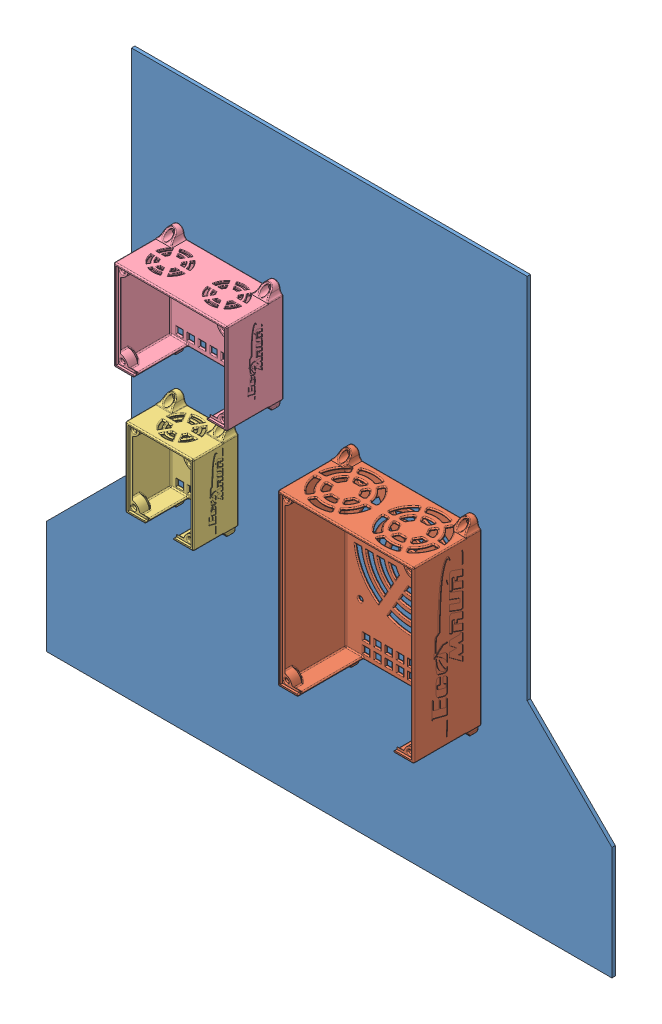
SolidWorks assembly placa_suporte_eletronica_montada, configuration Default. Lengths in mm.
Overall size (500 500 63).
4 component instances, 4 part files, 6 mates.
Components (placement in the parent):
- placa_suporte_eletronica-1: placa_suporte_eletronica [Default] at (-46.9137 -242.0268 17.8389) size (500 500 3)
- caixa_eco_ctrl_eletrico-1: caixa_eco_ctrl_eletrico [Default] at (27.6777 -30.9013 22.8389) x (0 -1 0) z (-1 0 0) size (167.5 60.1 120.01)
- caixa_eco_ctrl_acoplamento-1: caixa_eco_ctrl_acoplamento [Default] at (-157.1447 -25.5387 22.8389) x (0 -1 0) z (-1 0 0) size (87.5 40 60)
- caixa_eco_tx_telemetry-1: caixa_eco_tx_telemetry [Default] at (-137.4558 96.1278 22.8389) x (0 -1 0) z (-1 0 0) size (97.5 50 100)
Mates (geometry in assembly coordinates):
- Coincident1: coincident anti-aligned: plane of placa_suporte_eletronica-1 through (-46.9137 -242.0268 20.8389) normal (0 0 1); plane of caixa_eco_ctrl_eletrico-1 through (27.6777 -30.9013 20.8389) normal (0 0 -1)
- Coincident2: coincident anti-aligned: plane of placa_suporte_eletronica-1 through (-46.9137 -242.0268 20.8389) normal (0 0 1); plane of caixa_eco_tx_telemetry-1 through (-137.4558 96.1278 20.8389) normal (0 0 -1)
- Coincident3: coincident anti-aligned: plane of placa_suporte_eletronica-1 through (-46.9137 -242.0268 20.8389) normal (0 0 1); plane of caixa_eco_ctrl_acoplamento-1 through (-157.1447 -25.5387 20.8389) normal (0 0 -1)
- Parallel1: parallel aligned: plane of placa_suporte_eletronica-1 through (-221.9137 257.9732 20.8389) normal (0 1 0); plane of caixa_eco_ctrl_acoplamento-1 through (-157.1447 9.4613 20.8389) normal (0 1 0)
- Parallel2: parallel aligned: plane of placa_suporte_eletronica-1 through (-221.9137 257.9732 20.8389) normal (0 1 0); plane of caixa_eco_tx_telemetry-1 through (-137.4558 136.1278 20.8389) normal (0 1 0)
- Parallel3: parallel aligned: plane of placa_suporte_eletronica-1 through (-221.9137 257.9732 20.8389) normal (0 1 0); plane of caixa_eco_ctrl_eletrico-1 through (27.6777 44.0987 20.8389) normal (0 1 0)
